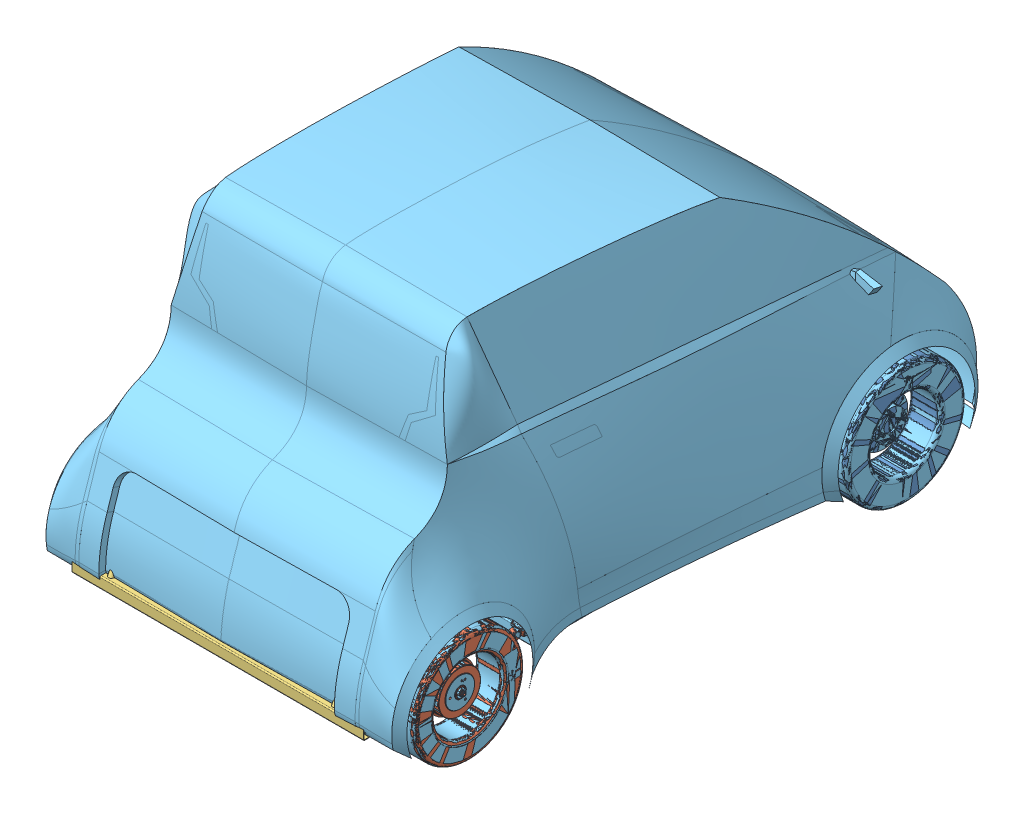
SolidWorks assembly 22aug, configuration Default. Lengths in mm.
Overall size (5751.02 1566.72 2786.51).
5 component instances, 5 part files, 12 mates.
Components (placement in the parent):
- FRONT POINTS PART-1: FRONT POINTS PART [Default] at (-4821.3196 268.4 428.9437) x (0 0 1) z (0 1 0) size (536.8 1560.65 826.66)
- REAR POINTS PART-1: REAR POINTS PART [Default] at (-4823.2763 246.9 2398.8264) x (1 0 0) z (0 1 0) size (1602.73 665.76 585.82)
- 21 08 chassis-1: 21 08 chassis [Default<As Machined>] at (-4821.6427 190.9138 157.369) x (0 0 1) z (-1 0 0) size (2580 626.85 1330)
- cockpit_trial 2-2: cockpit_trial 2 [Default<As Machined>] at (-4821.3105 230.9138 739.5219) x (-1 0 0) z (0 -1 0) size (1333.7 1641.85 1229.73)
- 12sep-1: 12sep [Default] at (-4821.2749 0 1392.0201) size (1859.5 1490.79 2786.51)
Mates (geometry in assembly coordinates):
- Tangent2: tangent anti-aligned: cylinder of FRONT POINTS PART-1 through (-4185.9966 268.4 428.9437) axis (1 0 0) radius 268.4; plane of assembly through (0 0 0) normal (0 1 0)
- Parallel1: parallel anti-aligned: plane of FRONT POINTS PART-1 through (-5601.6427 268.4 428.9437) normal (-1 0 0); plane of assembly through (0 0 0) normal (1 0 0)
- Tangent3: tangent anti-aligned: cylinder of REAR POINTS PART-1 through (-5487.6427 246.9 2398.8264) axis (-1 0 0) radius 246.9; plane of assembly through (0 0 0) normal (0 1 0)
- Parallel2: parallel aligned: plane of FRONT POINTS PART-1; plane of assembly through (0 0 0) normal (0 0 1)
- Parallel3: parallel anti-aligned: plane of REAR POINTS PART-1 through (-4823.2763 246.9 2398.8264) normal (0 0 -1); plane of assembly through (0 0 0) normal (0 0 1)
- Distance1: distance = 1970 mm: axis of FRONT POINTS PART-1 through (-5476.6427 268.4 428.9437) axis (-1 0 0); axis of REAR POINTS PART-1 through (-5742.3677 246.9 2398.8264) axis (1 0 0)
- Distance2: distance = 21 mm aligned: plane of FRONT POINTS PART-1 through (-5601.6427 268.4 428.9437) normal (-1 0 0); plane of REAR POINTS PART-1 through (-5622.6427 246.9 2398.8264) normal (-1 0 0)
- Distance5: distance = 14 mm aligned: plane of 21 08 chassis-1 through (-5101.8427 215.9138 757.369) normal (0 1 0); plane of FRONT POINTS PART-1 through (-5154.4031 201.9138 420.1608) normal (0 1 0)
- Distance6: distance = 115 mm aligned: plane of 21 08 chassis-1 through (-5486.6427 210.7138 757.369) normal (-1 0 0); plane of FRONT POINTS PART-1 through (-5601.6427 268.4 428.9437) normal (-1 0 0)
- Coincident8: coincident aligned: plane of FRONT POINTS PART-1 through (-5601.6427 268.4 428.9437) normal (-1 0 0); plane of 12sep-1 through (-5601.6427 268.4 428.9437) normal (-1 0 0)
- Concentric1: concentric aligned: cylinder of FRONT POINTS PART-1 through (-5456.6427 268.4 428.9437) axis (-1 0 0) radius 268.4; cylinder of 12sep-1 through (-5456.6427 268.4 428.9437) axis (-1 0 0) radius 268.4
- Coincident9: coincident anti-aligned: plane of 21 08 chassis-1 through (-4161.8427 215.9138 1957.369) normal (0 1 0); plane of cockpit_trial 2-2 through (-4181.1105 215.9138 1919.5219) normal (0 -1 0)
